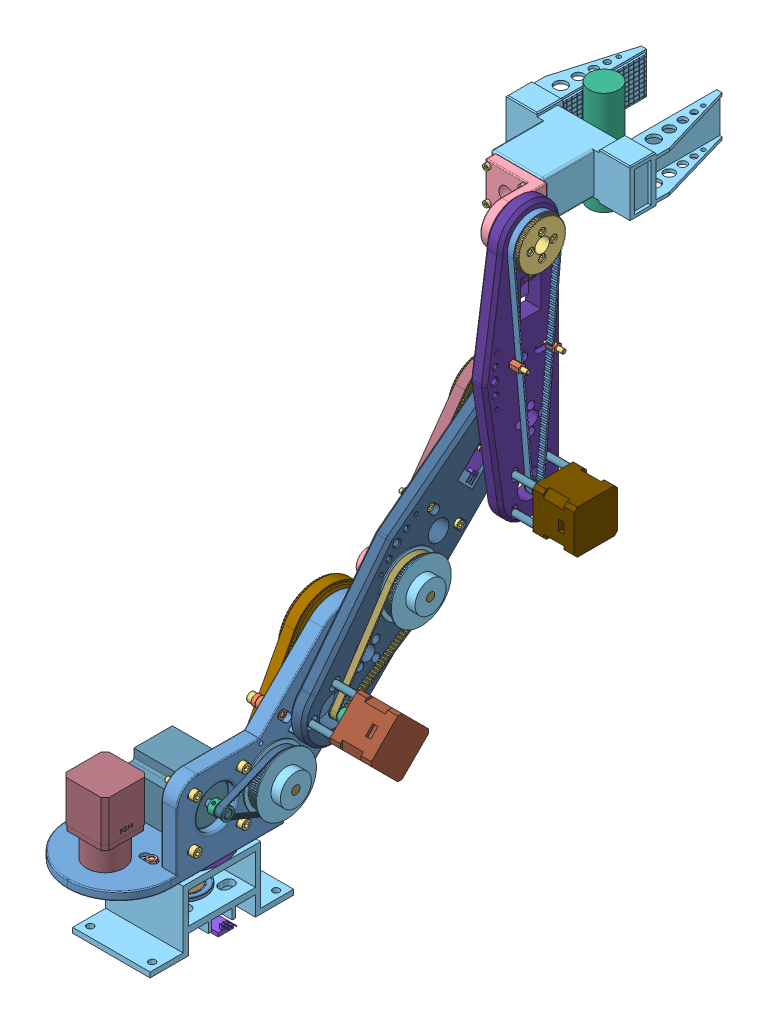
SolidWorks assembly R4 assem home axis, configuration Default. Lengths in mm.
Overall size (201 534.19 555.69).
175 component instances, 42 part files, 380 mates.
Components (placement in the parent):
- arm1-1: arm1 [Default] at (0 22.25 32) x (0 0 1) z (0 1 0) size (257.74 100 155.28)
- bearingCover-1: bearingCover [Default] at (50 142.4912 -110.7437) x (0 -0.707107 -0.707107) z (1 0 0) size (32 32 3)
- shaftJ1-1: shaftJ1 [Default] at (0 -34.75 0) x (0 0 -1) z (1 0 0) size (50 69 50)
- Pulleyhtd3m20Tbore8-1: Pulleyhtd3m20Tbore8 [Default] at (0 12.5 75.6) x (1 0 0) z (0 -1 0) size (22 22 24)
- pulley2GT80T-1: pulley2GT80T [Default] at (57.6 67.75 -36.0025) x (0 -0.778145 -0.628085) z (1 0 0) size (58 58 22)
- pulley2GT16Tbore6.35-1: pulley2GT16Tbore6.35 [Default] at (56.1 67.75 17.0975) x (0 0.483708 -0.87523) z (1 0 0) size (12.2 12.2 14)
- PulleyHTD3m15Tbore8-1: PulleyHTD3m15Tbore8 [Default] at (26.5 67.75 -36.0025) x (0 0.57686 0.816843) z (1 0 0) size (14 14 19.5)
- BeltHTD3m312L20T80T-1: BeltHTD3m312L20T80T [Default] at (0 12.5 0) x (0 0 1) z (0 1 0) size (125.04 78.09 10)
- BeltHTD3m363L15T80T-1: BeltHTD3m363L15T80T [Default] at (26.5 142.4912 -110.7437) x (0 -0.707107 0.707107) z (-1 0 0) size (152.76 78.09 10)
- belt2GT210L-1: belt2GT210L [Default] at (56.1 67.75 17.0975) x (0 0 -1) z (1 0 0) size (84.41 51.68 6)
- MagneticSensorV2-2: MagneticSensorV2 [Default] at (45.9 115.6211 -83.8737) x (0 -0.707107 0.707107) z (1 0 0) size (31 15 9)
- shaft8x70-1: shaft8x70 [Default] at (73.1 67.75 -36.0025) x (0 0 1) z (-1 0 0) size (8 8 61)
- Nema17L40PG14-1: Nema17L40PG14 [Default] at (0 99.75 75.6) x (0 0 -1) z (0 -1 0) size (42 42 88.5)
- Nema23_57x57x56-2: Nema23_57x57x56 [Default] at (-12 67.75 17.0975) x (0 0 -1) z (1 0 0) size (57 57 73)
- BeltTensionSpacer-1: BeltTensionSpacer [Default] at (35 113.7119 -46.6091) x (0 -0.41678 -0.909008) z (-1 0 0) size (6.4 6.4 3)
- BeltTensionSpacer-2: BeltTensionSpacer [Default] at (35 78.3566 -81.9645) x (0 -0.41678 -0.909008) z (-1 0 0) size (6.4 6.4 3)
- BeltTensionSpacer-6: BeltTensionSpacer [Default] at (-24.5 19.25 55) x (0.999608 0 0.027999) z (0 1 0) size (6.4 6.4 3)
- BeltTensionSpacer-5: BeltTensionSpacer [Default] at (24.5 22.25 55) x (0.852155 0 0.52329) z (0 -1 0) size (6.4 6.4 3)
- Washer45x60x1-2: Washer45x60x1 [5909K79] at (0 22.25 0) x (0 -1 0) z (0.730209 0 -0.683224) size (1 65 65)
- Washer45x60x1-1: Washer45x60x1 [5909K79] at (0 18.3 0) x (0 -1 0) z (0.528749 0 -0.848778) size (1 65 65)
- NeedleThrustBearing5909_45x60x3-1: NeedleThrustBearing5909_45x60x3 [5909K19] at (0 20.275 0) x (0.862783 0 0.505574) z (0.505574 0 -0.862783) size (65 3 65)
- bearing608 8x22x7-1: bearing608 8x22x7 [Default] at (50 67.75 -36.0025) x (0 -0.065699 -0.997839) z (0 0.997839 -0.065699) size (22 7 22)
- bearing608 8x22x7-2: bearing608 8x22x7 [Default] at (35 67.75 -36.0025) x (0 -0.995759 -0.092005) z (0 -0.092005 0.995759) size (22 7 22)
- bearing6806 30x42x7-3: bearing6806 30x42x7 [5972K282] at (38.5 142.4912 -110.7437) x (0 0.778145 0.628085) z (1 0 0) size (42 42 7)
- bearing6806 30x42x7-4: bearing6806 30x42x7 [5972K282] at (46.5 142.4912 -110.7437) x (0 -0.232241 -0.972658) z (-1 0 0) size (42 42 7)
- Bearing105 5x10x4-1: Bearing105 5x10x4 [7804K106] at (30 113.7119 -46.6091) x (0 0.558787 -0.829311) z (-1 0 0) size (10 10 4)
- Bearing105 5x10x4-4: Bearing105 5x10x4 [7804K106] at (26.1 78.3566 -81.9645) x (0 -0.623411 0.781894) z (-1 0 0) size (10 10 4)
- Bearing105 5x10x4-9: Bearing105 5x10x4 [7804K106] at (24.5 17.25 55) x (0.890608 0 -0.454771) z (0 -1 0) size (10 10 4)
- Bearing105 5x10x4-10: Bearing105 5x10x4 [7804K106] at (24.5 13.25 55) x (0.890608 0 -0.454771) z (0 -1 0) size (10 10 4)
- Bearing105 5x10x4-11: Bearing105 5x10x4 [7804K106] at (-24.5 13.25 55) x (-0.374722 0 0.927137) z (0 1 0) size (10 10 4)
- Bearing105 5x10x4-12: Bearing105 5x10x4 [7804K106] at (-24.5 17.25 55) x (0.156116 0 0.987739) z (0 1 0) size (10 10 4)
- Bearing105 5x10x4-2: Bearing105 5x10x4 [7804K106] at (26 113.7119 -46.6091) x (0 -0.774653 -0.632387) z (-1 0 0) size (10 10 4)
- Bearing105 5x10x4-3: Bearing105 5x10x4 [7804K106] at (30.1 78.3566 -81.9645) x (0 -0.931032 -0.364937) z (1 0 0) size (10 10 4)
- socket head cap screw_iso0-13: socket head cap screw_iso0 [ISO 4762 M4 x 12 - 12N] at (0 38.25 20) x (0 -1 0) z (0 0 1) size (16 7 7)
- socket head cap screw_iso0-14: socket head cap screw_iso0 [ISO 4762 M4 x 12 - 12N] at (20 38.25 0) x (0 -1 0) z (0 0 1) size (16 7 7)
- socket head cap screw_iso0-15: socket head cap screw_iso0 [ISO 4762 M4 x 12 - 12N] at (0 38.25 -20) x (0 -1 0) z (0 0 1) size (16 7 7)
- socket head cap screw_iso0-16: socket head cap screw_iso0 [ISO 4762 M4 x 12 - 12N] at (-20 38.25 0) x (0 -1 0) z (0 0 1) size (16 7 7)
- hex nut style 1 gradeab_iso00-1: hex nut style 1 gradeab_iso00 [ISO - 4032 - M5 - W - N] at (49.7 113.7119 -46.6091) x (0 -0.707107 0.707107) z (1 0 0) size (8 9.24 4.7)
- hex nut style 1 gradeab_iso00-2: hex nut style 1 gradeab_iso00 [ISO - 4032 - M5 - W - N] at (49.7 78.3566 -81.9645) x (0 0.965926 0.258819) z (1 0 0) size (8 9.24 4.7)
- socket head cap screw_iso0-20: socket head cap screw_iso0 [ISO 4762 M5 x 25 - 25N] at (19 113.7119 -46.6091) size (30 8.5 8.5)
- socket head cap screw_iso0-21: socket head cap screw_iso0 [ISO 4762 M5 x 25 - 25N] at (19.1 78.3566 -81.9645) size (30 8.5 8.5)
- socket head cap screw_iso0-57: socket head cap screw_iso0 [ISO 4762 M5 x 20 - 20N] at (24.5 6.25 55) x (0 1 0) z (0 0 1) size (25 8.5 8.5)
- socket head cap screw_iso0-58: socket head cap screw_iso0 [ISO 4762 M5 x 20 - 20N] at (-24.5 6.25 55) x (0 1 0) z (0 0 1) size (25 8.5 8.5)
- hex nut style 1 gradeab_iso00-15: hex nut style 1 gradeab_iso00 [ISO - 4032 - M5 - W - N] at (-24.5 31.95 55) x (-0.866025 0 0.5) z (0 1 0) size (8 9.24 4.7)
- hex nut style 1 gradeab_iso00-16: hex nut style 1 gradeab_iso00 [ISO - 4032 - M5 - W - N] at (24.5 31.95 55) x (-0.866025 0 -0.5) z (0 1 0) size (8 9.24 4.7)
- socket head cap screw_iso0-80: socket head cap screw_iso0 [ISO 4762 M2 x 12 - 12N] at (51.4 117.7424 -93.066) x (-1 0 0) z (0 0.924225 0.381849) size (14 3.8 3.8)
- socket head cap screw_iso0-81: socket head cap screw_iso0 [ISO 4762 M2 x 12 - 12N] at (51.4 124.8135 -85.995) x (-1 0 0) z (0 0.924225 0.381849) size (14 3.8 3.8)
- hex nut style 1 gradeab_iso00-25: hex nut style 1 gradeab_iso00 [ISO - 4032 - M2 - W - N] at (37.4 117.7424 -93.066) x (0 0 1) z (-1 0 0) size (4 4.62 1.6)
- hex nut style 1 gradeab_iso00-26: hex nut style 1 gradeab_iso00 [ISO - 4032 - M2 - W - N] at (37.4 124.8135 -85.995) x (0 0 1) z (-1 0 0) size (4 4.62 1.6)
- socket head cap screw_iso0-96: socket head cap screw_iso0 [ISO 4762 M5 x 25 - 25N] at (55 91.32 40.6675) x (-1 0 0) z (0 -0.924225 -0.381849) size (30 8.5 8.5)
- socket head cap screw_iso0-97: socket head cap screw_iso0 [ISO 4762 M5 x 25 - 25N] at (55 91.32 -6.4725) x (-1 0 0) z (0 -0.924225 -0.381849) size (30 8.5 8.5)
- socket head cap screw_iso0-98: socket head cap screw_iso0 [ISO 4762 M5 x 25 - 25N] at (55 44.18 -6.4725) x (-1 0 0) z (0 -0.924225 -0.381849) size (30 8.5 8.5)
- socket head cap screw_iso0-99: socket head cap screw_iso0 [ISO 4762 M5 x 25 - 25N] at (55 44.18 40.6675) x (-1 0 0) z (0 -0.924225 -0.381849) size (30 8.5 8.5)
- socket head cap screw_iso0-104: socket head cap screw_iso0 [ISO 4762 M3 x 12 - 12N] at (9.8995 19.25 85.4995) x (0 1 0) z (0 0 1) size (15 5.5 5.5)
- socket head cap screw_iso0-105: socket head cap screw_iso0 [ISO 4762 M3 x 12 - 12N] at (9.8995 19.25 65.7005) x (0 1 0) z (0 0 1) size (15 5.5 5.5)
- socket head cap screw_iso0-106: socket head cap screw_iso0 [ISO 4762 M3 x 12 - 12N] at (-9.8995 19.25 85.4995) x (0 1 0) z (0 0 1) size (15 5.5 5.5)
- socket head cap screw_iso0-107: socket head cap screw_iso0 [ISO 4762 M3 x 12 - 12N] at (-9.8995 19.25 65.7005) x (0 1 0) z (0 0 1) size (15 5.5 5.5)
- hex nut style 1 gradeab_iso00-35: hex nut style 1 gradeab_iso00 [ISO - 4032 - M5 - W - N] at (30.3 91.32 40.6675) x (0 0 1) z (-1 0 0) size (8 9.24 4.7)
- hex nut style 1 gradeab_iso00-36: hex nut style 1 gradeab_iso00 [ISO - 4032 - M5 - W - N] at (30.3 91.32 -6.4725) x (0 0 1) z (-1 0 0) size (8 9.24 4.7)
- hex nut style 1 gradeab_iso00-37: hex nut style 1 gradeab_iso00 [ISO - 4032 - M5 - W - N] at (30.3 44.18 -6.4725) x (0 0 1) z (-1 0 0) size (8 9.24 4.7)
- hex nut style 1 gradeab_iso00-38: hex nut style 1 gradeab_iso00 [ISO - 4032 - M5 - W - N] at (40.3966 44.18 40.6675) x (0 0 -1) z (1 0 0) size (8 9.24 4.7)
- base-1: base [Default] x (1 0 0) z (0 1 0) size (75 138.93 61)
- bearing6806 30x42x7-1: bearing6806 30x42x7 [5972K282] at (0 -30.5984 0) x (0.837169 0 0.546944) z (0 -1 0) size (42 42 7)
- pulleyHTD3m80Tbase-1: pulleyHTD3m80Tbase [Default] at (0 12 0) x (1 0 0) z (0 1 0) size (75.63 75.63 12)
- bearing6806 30x42x7-2: bearing6806 30x42x7 [5972K282] at (0 14.3 0) x (0.999895 0 -0.014508) z (0 1 0) size (42 42 7)
- shaftJ1endPlate-1: shaftJ1endPlate [Default] at (0 -34.75 0) x (0 0 -1) z (0 -1 0) size (40 40 6)
- MagneticSensor-3: MagneticSensor [Default] at (31.5 -49.5984 0) x (1 0 0) z (0 1 0) size (31 15 7.5)
- socket head cap screw_iso0-132: socket head cap screw_iso0 [ISO 4762 M5 x 16 - 16N] at (21 -5 -21) x (0 1 0) z (0 0 1) size (21 8.5 8.5)
- socket head cap screw_iso0-133: socket head cap screw_iso0 [ISO 4762 M5 x 16 - 16N] at (21 -5 21) x (0 1 0) z (0 0 1) size (21 8.5 8.5)
- socket head cap screw_iso0-134: socket head cap screw_iso0 [ISO 4762 M5 x 16 - 16N] at (-21 -5 21) x (0 1 0) z (0 0 1) size (21 8.5 8.5)
- socket head cap screw_iso0-135: socket head cap screw_iso0 [ISO 4762 M5 x 16 - 16N] at (-21 -5 -21) x (0 1 0) z (0 0 1) size (21 8.5 8.5)
- socket head cap screw_iso0-136: socket head cap screw_iso0 [ISO 4762 M3 x 16 - 16N] at (12.5 -43.75 0) x (0 1 0) z (0 0 1) size (19 5.5 5.5)
- socket head cap screw_iso0-137: socket head cap screw_iso0 [ISO 4762 M3 x 16 - 16N] at (0 -43.75 12.5) x (0 1 0) z (0 0 1) size (19 5.5 5.5)
- socket head cap screw_iso0-138: socket head cap screw_iso0 [ISO 4762 M3 x 16 - 16N] at (-12.5 -43.75 0) x (0 1 0) z (0 0 1) size (19 5.5 5.5)
- socket head cap screw_iso0-139: socket head cap screw_iso0 [ISO 4762 M3 x 16 - 16N] at (0 -43.75 -12.5) x (0 1 0) z (0 0 1) size (19 5.5 5.5)
- socket head cap screw_iso0-140: socket head cap screw_iso0 [ISO 4762 M2 x 12 - 12N] at (23.5 -51.5984 -5) x (0 1 0) z (-0.11823 0 0.992986) size (14 3.8 3.8)
- socket head cap screw_iso0-141: socket head cap screw_iso0 [ISO 4762 M2 x 12 - 12N] at (23.5 -51.5984 5) x (0 1 0) z (0 0 1) size (14 3.8 3.8)
- hex nut style 1 gradeab_iso00-59: hex nut style 1 gradeab_iso00 [ISO - 4032 - M2 - W - N] at (23.5 -40.9984 -5) x (1 0 0) z (0 1 0) size (4 4.62 1.6)
- hex nut style 1 gradeab_iso00-60: hex nut style 1 gradeab_iso00 [ISO - 4032 - M2 - W - N] at (23.5 -40.9984 5) x (1 0 0) z (0 1 0) size (4 4.62 1.6)
- socket head cap screw_iso0-142: socket head cap screw_iso0 [ISO 4762 M4 x 40 - 20N] at (19 134.713 -102.9655) size (44 7 7)
- socket head cap screw_iso0-143: socket head cap screw_iso0 [ISO 4762 M4 x 40 - 20N] at (19 134.713 -118.5219) size (44 7 7)
- socket head cap screw_iso0-144: socket head cap screw_iso0 [ISO 4762 M4 x 40 - 20N] at (19 150.2694 -118.5219) size (44 7 7)
- socket head cap screw_iso0-145: socket head cap screw_iso0 [ISO 4762 M4 x 40 - 20N] at (19 150.2694 -102.9655) size (44 7 7)
- PulleyHtd3m80Tbore8-2: PulleyHtd3m80Tbore8 [Default] at (25.5 142.4912 -110.7437) x (0 -0.707107 -0.707107) z (1 0 0) size (75.96 75.93 32)
- arm2-1: arm2 [Default] at (60.5 110.6714 -78.9239) x (0 0.707107 -0.707107) z (1 0 0) size (300.08 74.89 15.27)
- bearing6806 30x42x7-5: bearing6806 30x42x7 [5972K282] at (64.5 280.4336 -248.6861) x (0 -0.073672 -0.997283) z (1 0 0) size (42 42 7)
- bearing6806 30x42x7-6: bearing6806 30x42x7 [5972K282] at (56.5 280.4336 -248.6861) x (0 -0.383049 0.923728) z (-1 0 0) size (42 42 7)
- bearing608 8x22x7-3: bearing608 8x22x7 [Default] at (68 181.3255 -149.578) x (0 0 -1) z (0 1 0) size (22 7 22)
- bearing608 8x22x7-4: bearing608 8x22x7 [Default] at (60 181.3255 -149.578) x (0 0 -1) z (0 1 0) size (22 7 22)
- nema17L48arm2-1: nema17L48arm2 [Défaut] at (111 140.3699 -78.9239) x (-1 0 0) z (0 0.707107 -0.707107) size (63 42 42)
- pulley2GT16Tbore6.35-2: pulley2GT16Tbore6.35 [Default] at (72.5 110.6714 -78.9239) x (0 0.383049 -0.923728) z (-1 0 0) size (12.2 12.2 14)
- pulley2GT80T-2: pulley2GT80T [Default] at (74.5 181.3255 -149.578) x (0 -0.954986 -0.296652) z (1 0 0) size (58 58 22)
- belt2GTarm2-1: belt2GTarm2 [Default] at (72 110.6714 -78.9239) x (0 0.707107 -0.707107) z (1 0 0) size (131.74 52.19 6)
- shaft8x70-2: shaft8x70 [Default] at (29 181.3255 -149.578) x (0 0.563863 -0.825868) z (1 0 0) size (8 8 61)
- Pulleyhtd3m20Tbore8-2: Pulleyhtd3m20Tbore8 [Default] at (46.5 181.3255 -149.578) x (0 0 -1) z (1 0 0) size (22 22 24)
- beltHTD3marm2-1: beltHTD3marm2 [Default] at (47 280.4336 -248.6861) x (0 -0.707107 0.707107) z (1 0 0) size (184.35 67.59 10)
- MagneticSensor-6: MagneticSensor [Default] at (63 250.028 -218.2805) x (0 -0.707107 0.707107) z (1 0 0) size (31 15 7.5)
- cover nuts-1: cover nuts [Default] at (68 110.6714 -56.2965) x (0 -0.818287 -0.57481) z (1 0 0) size (6 6 23)
- cover nuts-2: cover nuts [Default] at (68 133.2988 -78.9239) x (0 0.708033 -0.706179) z (1 0 0) size (6 6 23)
- cover nuts-3: cover nuts [Default] at (68 88.044 -78.9239) x (0 -0.829446 -0.558587) z (1 0 0) size (6 6 23)
- cover nuts-4: cover nuts [Default] at (91 110.6714 -101.5513) x (0 0 1) z (-1 0 0) size (6 6 23)
- hex thin nut chamfered gradeab_iso-2: hex thin nut chamfered gradeab_iso [ISO - 4035 - M4 - N] at (50.8 233.411 -172.6721) x (0 0 1) z (-1 0 0) size (7 8.08 2.2)
- hex thin nut chamfered gradeab_iso-3: hex thin nut chamfered gradeab_iso [ISO - 4035 - M4 - N] at (48.6 233.411 -172.6721) x (0 0 1) z (-1 0 0) size (7 8.08 2.2)
- hex thin nut chamfered gradeab_iso-4: hex thin nut chamfered gradeab_iso [ISO - 4035 - M4 - N] at (46.4 233.411 -172.6721) x (0 0 1) z (-1 0 0) size (7 8.08 2.2)
- hex thin nut chamfered gradeab_iso-5: hex thin nut chamfered gradeab_iso [ISO - 4035 - M4 - N] at (44.2 233.411 -172.6721) x (0 0 1) z (-1 0 0) size (7 8.08 2.2)
- hex thin nut chamfered gradeab_iso-6: hex thin nut chamfered gradeab_iso [ISO - 4035 - M4 - N] at (42 233.411 -172.6721) x (0 0 1) z (-1 0 0) size (7 8.08 2.2)
- hex thin nut chamfered gradeab_iso-7: hex thin nut chamfered gradeab_iso [ISO - 4035 - M4 - N] at (50.8 204.4196 -201.6635) x (0 0 1) z (-1 0 0) size (7 8.08 2.2)
- hex thin nut chamfered gradeab_iso-8: hex thin nut chamfered gradeab_iso [ISO - 4035 - M4 - N] at (48.6 204.4196 -201.6635) x (0 0 1) z (-1 0 0) size (7 8.08 2.2)
- hex thin nut chamfered gradeab_iso-9: hex thin nut chamfered gradeab_iso [ISO - 4035 - M4 - N] at (46.4 204.4196 -201.6635) x (0 0 1) z (-1 0 0) size (7 8.08 2.2)
- hex thin nut chamfered gradeab_iso-10: hex thin nut chamfered gradeab_iso [ISO - 4035 - M4 - N] at (44.2 204.4196 -201.6635) x (0 0 1) z (-1 0 0) size (7 8.08 2.2)
- hex thin nut chamfered gradeab_iso-11: hex thin nut chamfered gradeab_iso [ISO - 4035 - M4 - N] at (42 204.4196 -201.6635) x (0 0 1) z (-1 0 0) size (7 8.08 2.2)
- hex thin nut chamfered gradeab_iso-12: hex thin nut chamfered gradeab_iso [ISO - 4035 - M2 - N] at (64.2 259.2204 -220.4018) x (0 0 -1) z (1 0 0) size (4 4.62 1.2)
- hex thin nut chamfered gradeab_iso-13: hex thin nut chamfered gradeab_iso [ISO - 4035 - M2 - N] at (64.2 252.1493 -227.4729) x (0 0 -1) z (1 0 0) size (4 4.62 1.2)
- socket head cap screw_iso0-174: socket head cap screw_iso0 [ISO 4762 M3 x 30 - 18N] at (55 110.6714 -56.2965) size (33 5.5 5.5)
- socket head cap screw_iso0-175: socket head cap screw_iso0 [ISO 4762 M3 x 30 - 18N] at (55 133.2988 -78.9239) size (33 5.5 5.5)
- socket head cap screw_iso0-176: socket head cap screw_iso0 [ISO 4762 M3 x 30 - 18N] at (55 88.044 -78.9239) x (1 0 0) z (0 -0.320522 -0.947241) size (33 5.5 5.5)
- socket head cap screw_iso0-177: socket head cap screw_iso0 [ISO 4762 M3 x 30 - 18N] at (55 110.6714 -101.5513) size (33 5.5 5.5)
- socket head cap screw_iso0-189: socket head cap screw_iso0 [ISO 4762 M4 x 25 - 25N] at (67 233.411 -172.6721) x (-1 0 0) z (0 0.247798 0.968812) size (29 7 7)
- socket head cap screw_iso0-190: socket head cap screw_iso0 [ISO 4762 M4 x 25 - 25N] at (67 204.4196 -201.6635) x (-1 0 0) z (0 -0.924225 -0.381849) size (29 7 7)
- socket head cap screw_iso0-191: socket head cap screw_iso0 [ISO 4762 M2 x 10 - 10N] at (68.5 259.2204 -220.4018) x (-1 0 0) z (0 0.924225 0.381849) size (12 3.8 3.8)
- socket head cap screw_iso0-192: socket head cap screw_iso0 [ISO 4762 M2 x 10 - 10N] at (68.5 252.1493 -227.4729) x (-1 0 0) z (0 0.924225 0.381849) size (12 3.8 3.8)
- hex thin nut chamfered gradeab_iso-14: hex thin nut chamfered gradeab_iso [ISO - 4035 - M2 - N] at (56.8 259.2204 -220.4018) x (0 0 1) z (-1 0 0) size (4 4.62 1.2)
- hex thin nut chamfered gradeab_iso-15: hex thin nut chamfered gradeab_iso [ISO - 4035 - M2 - N] at (56.8 252.1493 -227.4729) x (0 0 1) z (-1 0 0) size (4 4.62 1.2)
- socket head cap screw_iso0-193: socket head cap screw_iso0 [ISO 4762 M4 x 40 - 20N] at (39 269.4336 -248.6861) size (44 7 7)
- socket head cap screw_iso0-194: socket head cap screw_iso0 [ISO 4762 M4 x 40 - 20N] at (39 291.4336 -248.6861) size (44 7 7)
- socket head cap screw_iso0-195: socket head cap screw_iso0 [ISO 4762 M4 x 40 - 20N] at (39 280.4336 -237.6861) size (44 7 7)
- socket head cap screw_iso0-196: socket head cap screw_iso0 [ISO 4762 M4 x 40 - 20N] at (39 280.4336 -259.6861) size (44 7 7)
- PulleyHtd3m80Tbore8arm2-1: PulleyHtd3m80Tbore8arm2 [Default] at (45.5 280.4336 -248.6861) x (0 0 -1) z (1 0 0) size (63.51 63.51 32)
- bearingCover-2: bearingCover [Default] at (73 280.4336 -248.6861) x (0 -1 0) z (-1 0 0) size (32 32 3)
- arm3-1: arm3 [Default] at (80.5 225.4336 -248.6861) x (0 1 0) z (1 0 0) size (265.75 74.89 15.27)
- bearing6806 30x42x7-7: bearing6806 30x42x7 [5972K282] at (84.5 431.1836 -248.6861) x (0 0 -1) z (1 0 0) size (42 42 7)
- bearing6806 30x42x7-8: bearing6806 30x42x7 [5972K282] at (76.5 431.1836 -248.6861) x (0 0 -1) z (1 0 0) size (42 42 7)
- nema17L48arm3-1: nema17L48arm3 [Défaut] at (131 246.4336 -227.6861) x (-1 0 0) z (0 1 0) size (63 42 42)
- pulley2GT16Tbore6.35-3: pulley2GT16Tbore6.35 [Default] at (92.5 225.4336 -248.6861) x (0 0.383049 -0.923728) z (-1 0 0) size (12.2 12.2 14)
- belt2GTarm3-1: belt2GTarm3 [Default] at (92 431.1836 -248.6861) x (0 -1 0) z (1 0 0) size (235.46 47.53 6)
- MagneticSensor-4: MagneticSensor [Default] at (78 386.1836 -248.6861) x (0 -1 0) z (-1 0 0) size (31 15 7.5)
- cover nuts-5: cover nuts [Default] at (88 209.4336 -232.6861) x (0 -0.924225 -0.381849) z (1 0 0) size (6 6 23)
- cover nuts-6: cover nuts [Default] at (88 241.4336 -232.6861) x (0 -0.921224 -0.389031) z (1 0 0) size (6 6 23)
- cover nuts-7: cover nuts [Default] at (88 209.4336 -264.6861) x (0 -0.923758 -0.382976) z (1 0 0) size (6 6 23)
- cover nuts-8: cover nuts [Default] at (88 241.4336 -264.6861) x (0 -0.832631 -0.553828) z (1 0 0) size (6 6 23)
- socket head cap screw_iso0-197: socket head cap screw_iso0 [ISO 4762 M2 x 10 - 10N] at (72.5 394.1836 -243.6861) size (12 3.8 3.8)
- socket head cap screw_iso0-198: socket head cap screw_iso0 [ISO 4762 M2 x 10 - 10N] at (72.5 394.1836 -253.6861) size (12 3.8 3.8)
- hex thin nut gradeb_iso00-2: hex thin nut gradeb_iso00 [ISO - 4036 - M2 - N] at (84.2 394.1836 -243.6861) x (0 0 -1) z (1 0 0) size (4 4.62 1.2)
- hex thin nut gradeb_iso00-3: hex thin nut gradeb_iso00 [ISO - 4036 - M2 - N] at (84.2 394.1836 -253.6861) x (0 0 -1) z (1 0 0) size (4 4.62 1.2)
- hex thin nut gradeb_iso00-4: hex thin nut gradeb_iso00 [ISO - 4036 - M4 - N] at (90.2 334.9698 -231.3738) x (0 0 -1) z (1 0 0) size (7 8.08 2.2)
- hex thin nut gradeb_iso00-5: hex thin nut gradeb_iso00 [ISO - 4036 - M4 - N] at (92.4 334.9698 -231.3738) x (0 0 -1) z (1 0 0) size (7 8.08 2.2)
- hex thin nut gradeb_iso00-6: hex thin nut gradeb_iso00 [ISO - 4036 - M4 - N] at (94.6 334.9698 -231.3738) x (0 0 -1) z (1 0 0) size (7 8.08 2.2)
- hex thin nut gradeb_iso00-7: hex thin nut gradeb_iso00 [ISO - 4036 - M4 - N] at (96.8 334.9698 -231.3738) x (0 0 -1) z (1 0 0) size (7 8.08 2.2)
- hex thin nut gradeb_iso00-8: hex thin nut gradeb_iso00 [ISO - 4036 - M4 - N] at (90.2 334.9698 -266.1861) x (0 0 -1) z (1 0 0) size (7 8.08 2.2)
- hex thin nut gradeb_iso00-9: hex thin nut gradeb_iso00 [ISO - 4036 - M4 - N] at (92.4 334.9698 -266.1861) x (0 0 -1) z (1 0 0) size (7 8.08 2.2)
- hex thin nut gradeb_iso00-10: hex thin nut gradeb_iso00 [ISO - 4036 - M4 - N] at (94.6 334.9698 -266.1861) x (0 0 -1) z (1 0 0) size (7 8.08 2.2)
- hex thin nut gradeb_iso00-11: hex thin nut gradeb_iso00 [ISO - 4036 - M4 - N] at (96.8 334.9698 -266.1861) x (0 0 -1) z (1 0 0) size (7 8.08 2.2)
- socket head cap screw_iso0-199: socket head cap screw_iso0 [ISO 4762 M3 x 30 - 18N] at (75 209.4336 -232.6861) size (33 5.5 5.5)
- socket head cap screw_iso0-200: socket head cap screw_iso0 [ISO 4762 M3 x 30 - 18N] at (75 241.4336 -232.6861) size (33 5.5 5.5)
- socket head cap screw_iso0-201: socket head cap screw_iso0 [ISO 4762 M3 x 30 - 18N] at (75 209.4336 -264.6861) x (1 0 0) z (0 -0.331782 0.943356) size (33 5.5 5.5)
- socket head cap screw_iso0-202: socket head cap screw_iso0 [ISO 4762 M3 x 30 - 18N] at (75 241.4336 -264.6861) x (1 0 0) z (0 -0.017552 0.999846) size (33 5.5 5.5)
- socket head cap screw_iso0-203: socket head cap screw_iso0 [ISO 4762 M4 x 25 - 25N] at (74 334.9698 -231.3738) x (1 0 0) z (0 0.99119 0.132448) size (29 7 7)
- socket head cap screw_iso0-204: socket head cap screw_iso0 [ISO 4762 M4 x 25 - 25N] at (74 334.9698 -266.1861) x (1 0 0) z (0 -0.279125 0.960255) size (29 7 7)
- pulley2GT60T-1: pulley2GT60T [Default] at (93.5 431.1836 -248.6861) x (0 0 1) z (-1 0 0) size (45.3 45.3 27)
- gripper holder-1: gripper holder [Default] at (64 431.1836 -248.6861) x (0 0 -1) z (1 0 0) size (55 40 50)
- Part1g-1: Part1g [Default] at (39.0001 431.1835 -283.6861) x (1 -0.000137 0) z (0 0 1) size (120 46 160)
- payload-1: payload [Default] at (39.493 379.1834 -368.0651) x (0.990185 -0.000136 -0.139766) z (0.000137 1 0) size (28.76 28.76 100)
- bearingCover-3: bearingCover [Default] at (72 431.1836 -248.6861) x (0 -1 0) z (-1 0 0) size (32 32 3)
- hex thin nut gradeb_iso00-12: hex thin nut gradeb_iso00 [ISO - 4036 - M4 - N] at (56.8 442.1836 -248.6861) x (0 0 1) z (-1 0 0) size (7 8.08 2.2)
- hex thin nut gradeb_iso00-13: hex thin nut gradeb_iso00 [ISO - 4036 - M4 - N] at (56.8 420.1836 -248.6861) x (0 0 1) z (-1 0 0) size (7 8.08 2.2)
- hex thin nut gradeb_iso00-14: hex thin nut gradeb_iso00 [ISO - 4036 - M4 - N] at (56.8 431.1836 -237.6861) x (0 0 1) z (-1 0 0) size (7 8.08 2.2)
- hex thin nut gradeb_iso00-15: hex thin nut gradeb_iso00 [ISO - 4036 - M4 - N] at (56.8 431.1836 -259.6861) x (0 0 1) z (-1 0 0) size (7 8.08 2.2)
- socket head cap screw_iso0-205: socket head cap screw_iso0 [ISO 4762 M3 x 20 - 20N] at (56.22 446.6859 -270.6861) x (0 0 -1) z (0.996957 -0.077948 0) size (23 5.5 5.5)
- socket head cap screw_iso0-206: socket head cap screw_iso0 [ISO 4762 M3 x 20 - 20N] at (21.78 415.6813 -270.6861) x (0 0 -1) z (0.996957 -0.077948 0) size (23 5.5 5.5)
- socket head cap screw_iso0-207: socket head cap screw_iso0 [ISO 4762 M3 x 20 - 20N] at (21.78 446.6859 -270.6861) x (0 0 -1) z (0.996957 -0.077948 0) size (23 5.5 5.5)
- socket head cap screw_iso0-208: socket head cap screw_iso0 [ISO 4762 M3 x 20 - 20N] at (56.22 415.6813 -270.6861) x (0 0 -1) z (0.996957 -0.077948 0) size (23 5.5 5.5)
- socket head cap screw_iso0-209: socket head cap screw_iso0 [ISO 4762 M4 x 35 - 20N] at (98 442.1836 -248.6861) x (-1 0 0) z (0 0.924225 0.381849) size (39 7 7)
- socket head cap screw_iso0-210: socket head cap screw_iso0 [ISO 4762 M4 x 35 - 20N] at (98 420.1836 -248.6861) x (-1 0 0) z (0 0.924225 0.381849) size (39 7 7)
- socket head cap screw_iso0-211: socket head cap screw_iso0 [ISO 4762 M4 x 35 - 20N] at (98 431.1836 -237.6861) x (-1 0 0) z (0 0.924225 0.381849) size (39 7 7)
- socket head cap screw_iso0-212: socket head cap screw_iso0 [ISO 4762 M4 x 35 - 20N] at (98 431.1836 -259.6861) x (-1 0 0) z (0 0.924225 0.381849) size (39 7 7)
Mates (geometry in assembly coordinates):
- Fix J1: parallel aligned: plane of base-1 through (37.5 6 37.5) normal (1 0 0); plane of arm1-1 through (50 30.25 -48) normal (1 0 0)
- Concentric1: concentric aligned: cylinder of base-1 through (0 29.44 0) axis (0 -1 0) radius 21.05; cylinder of bearing6806 30x42x7-1 through (0 -34.0984 0) axis (0 -1 0) radius 21
- Coincident1: coincident anti-aligned: plane of base-1 through (0 -34.0984 0) normal (0 1 0); plane of bearing6806 30x42x7-1 through (-11.2944 -34.0984 17.2875) normal (0 -1 0)
- Concentric2: concentric anti-aligned: cylinder of base-1 through (0 6 0) axis (0 -1 0) radius 16; cylinder of pulleyHTD3m80Tbase-1 through (0 10.8 0) axis (0 1 0) radius 21.05
- Concentric3: concentric anti-aligned: cylinder of base-1 through (21 6 21) axis (0 -1 0) radius 2.75; cylinder of pulleyHTD3m80Tbase-1 through (21 6 21) axis (0 1 0) radius 3
- Coincident2: coincident anti-aligned: plane of base-1 through (0 6 0) normal (0 1 0); plane of pulleyHTD3m80Tbase-1 through (0 6 0) normal (0 -1 0)
- Concentric4: concentric aligned: cylinder of base-1 through (21 6 -21) axis (0 -1 0) radius 2.75; cylinder of socket head cap screw_iso-1 through (21 -36.75 -21) axis (0 -1 0) radius 4.25
- Coincident3: coincident anti-aligned: plane of base-1 through (0 0 0) normal (0 -1 0); plane of socket head cap screw_iso-1 through (16.75 0 -21) normal (0 1 0)
- Concentric5: concentric aligned: cylinder of base-1 through (21 6 21) axis (0 -1 0) radius 2.75; cylinder of socket head cap screw_iso-2 through (21 -36.75 21) axis (0 -1 0) radius 4.25
- Coincident4: coincident anti-aligned: plane of base-1 through (0 0 0) normal (0 -1 0); plane of socket head cap screw_iso-2 through (16.75 0 21) normal (0 1 0)
- Concentric6: concentric aligned: cylinder of base-1 through (-21 6 21) axis (0 -1 0) radius 2.75; cylinder of socket head cap screw_iso-3 through (-21 -36.75 21) axis (0 -1 0) radius 4.25
- Coincident5: coincident anti-aligned: plane of base-1 through (0 0 0) normal (0 -1 0); plane of socket head cap screw_iso-3 through (-25.25 0 21) normal (0 1 0)
- Concentric7: concentric aligned: cylinder of base-1 through (-21 6 -21) axis (0 -1 0) radius 2.75; cylinder of socket head cap screw_iso-4 through (-21 -36.75 -21) axis (0 -1 0) radius 4.25
- Coincident6: coincident anti-aligned: plane of base-1 through (0 0 0) normal (0 -1 0); plane of socket head cap screw_iso-4 through (-25.25 0 -21) normal (0 1 0)
- Concentric8: concentric aligned: cylinder of pulleyHTD3m80Tbase-1 through (0 10.8 0) axis (0 1 0) radius 21.05; cylinder of bearing6806 30x42x7-2 through (0 17.8 0) axis (0 1 0) radius 21
- Coincident7: coincident anti-aligned: plane of pulleyHTD3m80Tbase-1 through (0 10.8 0) normal (0 1 0); plane of bearing6806 30x42x7-2 through (-0.2996 10.8 -20.6478) normal (0 -1 0)
- Concentric9: concentric aligned: cylinder of pulleyHTD3m80Tbase-1 through (0 10.8 0) axis (0 1 0) radius 21.05; cylinder of Washer45x60x1-1 through (0 17.8 0) axis (0 1 0) radius 32.5
- Coincident8: coincident anti-aligned: plane of pulleyHTD3m80Tbase-1 through (0 17.8 0) normal (0 1 0); plane of Washer45x60x1-1 through (0 17.8 0) normal (0 -1 0)
- Concentric10: concentric anti-aligned: cylinder of pulleyHTD3m80Tbase-1 through (0 10.8 0) axis (0 1 0) radius 21.05; cylinder of NeedleThrustBearing5909_45x60x3-1 through (0 18.775 0) axis (0 -1 0) radius 32.5
- Distance1: distance = 0.2 mm anti-aligned: plane of NeedleThrustBearing5909_45x60x3-1 through (-16.4311 19 28.0405) normal (0 -1 0); plane of Washer45x60x1-1 through (0 18.8 0) normal (0 1 0)
- Concentric11: concentric aligned: cylinder of pulleyHTD3m80Tbase-1 through (0 10.8 0) axis (0 1 0) radius 21.05; cylinder of Washer45x60x1-2 through (0 21.75 0) axis (0 1 0) radius 22.525
- Distance2: distance = 0.2 mm anti-aligned: plane of NeedleThrustBearing5909_45x60x3-1 through (-16.2626 21.55 27.7529) normal (0 1 0); plane of Washer45x60x1-2 through (0 21.75 0) normal (0 -1 0)
- Concentric12: concentric aligned: cylinder of base-1 through (0 6 0) axis (0 -1 0) radius 16; cylinder of arm1-1 through (0 30.25 0) axis (0 -1 0) radius 15.5
- Coincident12: coincident anti-aligned: plane of arm1-1 through (0 22.75 0) normal (0 -1 0); plane of Washer45x60x1-2 through (0 22.75 0) normal (0 1 0)
- Concentric15: concentric anti-aligned: cylinder of arm1-1 through (0 30.25 75.6) axis (0 -1 0) radius 11.5; cylinder of Nema17L40PG14-1 through (0 30.25 75.6) axis (0 1 0) radius 18
- Concentric16: concentric aligned: cylinder of arm1-1 through (-9.8995 30.25 85.4995) axis (0 -1 0) radius 1.65; cylinder of Nema17L40PG14-1 through (-9.8995 38.25 85.4995) axis (0 -1 0) radius 2
- Coincident16: coincident anti-aligned: plane of arm1-1 through (0 30.25 32) normal (0 1 0); plane of Nema17L40PG14-1 through (0 30.25 75.6) normal (0 -1 0)
- Concentric20: concentric anti-aligned: cylinder of Nema17L40PG14-1 through (0 11.25 75.6) axis (0 1 0) radius 4; cylinder of Pulleyhtd3m20Tbore8-1 through (0 30 75.6) axis (0 -1 0) radius 11
- Coincident17: coincident anti-aligned: plane of pulleyHTD3m80Tbase-1 through (0 18 0) normal (0 1 0); plane of Pulleyhtd3m20Tbore8-1 through (0 18 75.6) normal (0 -1 0)
- Concentric21: concentric aligned: cylinder of NeedleThrustBearing5909_45x60x3-1 through (0 18.775 0) axis (0 -1 0) radius 32.5; cylinder of BeltHTD3m312L20T80T-1 through (0 17.5 0) axis (0 -1 0) radius 39.0462
- Concentric22: concentric aligned: cylinder of Pulleyhtd3m20Tbore8-1 through (0 30 75.6) axis (0 -1 0) radius 11; cylinder of BeltHTD3m312L20T80T-1 through (0 17.5 75.6) axis (0 -1 0) radius 10.3983
- Distance3: distance = 0.5 mm anti-aligned: plane of Pulleyhtd3m20T-1 through (0 18 75.6) normal (0 -1 0); plane of BeltHTD3m312L20T80T-1 through (0 17.5 0) normal (0 1 0)
- Concentric23: concentric aligned: cylinder of arm1-1 through (0 30.25 0) axis (0 -1 0) radius 15.5; cylinder of shaftJ1-1 through (0 30.25 0) axis (0 -1 0) radius 15
- Concentric24: concentric aligned: cylinder of arm1-1 through (0 30.25 20) axis (0 -1 0) radius 2.75; cylinder of shaftJ1-1 through (0 34.25 20) axis (0 -1 0) radius 2.25
- Coincident19: coincident anti-aligned: plane of arm1-1 through (0 30.25 32) normal (0 1 0); plane of shaftJ1-1 through (0 30.25 0) normal (0 -1 0)
- Coincident24: coincident anti-aligned: plane of shaftJ1-1 through (0 -34.75 0) normal (0 -1 0); plane of shaftJ1endPlate-1 through (0 -34.75 0) normal (0 1 0)
- Concentric29: concentric anti-aligned: cylinder of shaftJ1-1 through (0 -14.75 12.5) axis (0 -1 0) radius 1.4; cylinder of shaftJ1endPlate-1 through (0 -40.75 12.5) axis (0 1 0) radius 1.75
- Concentric36: concentric anti-aligned: cylinder of shaftJ1-1 through (0 34.25 20) axis (0 -1 0) radius 2.25; cylinder of socket head cap screw_iso1-13 through (0 70 20) axis (0 1 0) radius 3.5
- Coincident31: coincident anti-aligned: plane of shaftJ1-1 through (0 34.25 0) normal (0 1 0); plane of socket head cap screw_iso1-13 through (3.5 34.25 20) normal (0 -1 0)
- Concentric37: concentric anti-aligned: cylinder of shaftJ1-1 through (20 34.25 0) axis (0 -1 0) radius 2.25; cylinder of socket head cap screw_iso1-14 through (20 70 0) axis (0 1 0) radius 3.5
- Coincident32: coincident anti-aligned: plane of shaftJ1-1 through (0 34.25 0) normal (0 1 0); plane of socket head cap screw_iso1-14 through (23.5 34.25 0) normal (0 -1 0)
- Concentric38: concentric anti-aligned: cylinder of shaftJ1-1 through (0 34.25 -20) axis (0 -1 0) radius 2.25; cylinder of socket head cap screw_iso1-15 through (0 70 -20) axis (0 1 0) radius 3.5
- Coincident33: coincident anti-aligned: plane of shaftJ1-1 through (0 34.25 0) normal (0 1 0); plane of socket head cap screw_iso1-15 through (3.5 34.25 -20) normal (0 -1 0)
- Concentric39: concentric anti-aligned: cylinder of shaftJ1-1 through (-20 34.25 0) axis (0 -1 0) radius 2.25; cylinder of socket head cap screw_iso1-16 through (-20 70 0) axis (0 1 0) radius 3.5
- Coincident34: coincident anti-aligned: circle of shaftJ1-1; plane of socket head cap screw_iso1-16 through (-16.5 34.25 0) normal (0 -1 0)
- Concentric41: concentric anti-aligned: cylinder of arm1-1 through (35 67.75 17.0975) axis (1 0 0) radius 19.5; cylinder of Nema23_57x57x56-2 through (61 67.75 17.0975) axis (-1 0 0) radius 3.175
- Coincident36: coincident anti-aligned: plane of arm1-1 through (40 22.25 32) normal (-1 0 0); plane of Nema23_57x57x56-2 through (40 67.75 17.0975) normal (1 0 0)
- Parallel2: parallel aligned: plane of arm1-1 through (35 105.25 55.9949) normal (0 1 0); plane of Nema23_57x57x56-2 through (40 96.25 45.5975) normal (0 1 0)
- Concentric42: concentric anti-aligned: cylinder of pulley2GT16Tbore6.35-1 through (46.6 67.75 17.0975) axis (1 0 0) radius 6.1; cylinder of Nema23_57x57x56-2 through (61 67.75 17.0975) axis (-1 0 0) radius 3.175
- Concentric43: concentric aligned: cylinder of arm1-1 through (43 67.75 -36.0025) axis (1 0 0) radius 11.05; cylinder of bearing608 8x22x7-1 through (43 67.75 -36.0025) axis (1 0 0) radius 11
- Coincident41: coincident anti-aligned: plane of arm1-1 through (43 67.75 -36.0025) normal (1 0 0); plane of bearing608 8x22x7-1 through (43 67.75 -36.0025) normal (-1 0 0)
- Concentric44: concentric aligned: cylinder of arm1-1 through (42 67.75 -36.0025) axis (-1 0 0) radius 11.05; cylinder of bearing608 8x22x7-2 through (42 67.75 -36.0025) axis (-1 0 0) radius 11
- Coincident42: coincident anti-aligned: plane of arm1-1 through (42 67.75 -36.0025) normal (-1 0 0); plane of bearing608 8x22x7-2 through (42 67.75 -36.0025) normal (1 0 0)
- Concentric45: concentric anti-aligned: cylinder of arm1-1 through (43 142.4912 -110.7437) axis (1 0 0) radius 21.05; cylinder of bearing6806 30x42x7-4 through (43 142.4912 -110.7437) axis (-1 0 0) radius 21
- Coincident43: coincident anti-aligned: plane of arm1-1 through (43 142.4912 -110.7437) normal (1 0 0); plane of bearing6806 30x42x7-4 through (43 122.4058 -105.9479) normal (-1 0 0)
- Concentric46: concentric anti-aligned: cylinder of arm1-1 through (42 142.4912 -110.7437) axis (-1 0 0) radius 21.05; cylinder of bearing6806 30x42x7-3 through (42 142.4912 -110.7437) axis (1 0 0) radius 21
- Coincident44: coincident anti-aligned: plane of arm1-1 through (42 142.4912 -110.7437) normal (-1 0 0); plane of bearing6806 30x42x7-3 through (42 129.5212 -94.675) normal (1 0 0)
- Concentric47: concentric aligned: cylinder of bearing608 8x22x7-1 through (43 67.75 -36.0025) axis (1 0 0) radius 4; cylinder of pulley2GT80T-1 through (51.1 67.75 -36.0025) axis (1 0 0) radius 4
- Distance4: distance = 0.5 mm aligned: plane of pulley2GT16Tbore6.35-1 through (52.6 67.75 17.0975) normal (1 0 0); plane of pulley2GT80Tbore8-1 through (52.1 67.75 -36.0025) normal (1 0 0)
- Concentric48: concentric anti-aligned: cylinder of bearing608 8x22x7-2 through (42 67.75 -36.0025) axis (-1 0 0) radius 4; cylinder of shaft8x70-1 through (12.1 67.75 -36.0025) axis (1 0 0) radius 4
- Coincident46: coincident aligned: plane of pulley2GT80T-1 through (73.1 67.75 -36.0025) normal (1 0 0); plane of shaft8x70-1 through (73.1 67.75 -36.0025) normal (1 0 0)
- disPulley1J1: distance = 5 mm anti-aligned: plane of pulley2GT16Tbore6.35-1 through (46.6 67.75 17.0975) normal (-1 0 0); plane of Nema23_57x57x56-2 through (41.6 67.75 17.0975) normal (1 0 0)
- Concentric51: concentric aligned: cylinder of pulley2GT80T-1 through (73.1 67.75 -36.0025) axis (-1 0 0) radius 15; cylinder of belt2GT210L-1 through (59.1 67.75 -36.0025) axis (-1 0 0) radius 25.84
- Concentric52: concentric anti-aligned: cylinder of pulley2GT16Tbore6.35-1 through (46.6 67.75 17.0975) axis (1 0 0) radius 6.1; cylinder of belt2GT210L-1 through (59.1 67.75 17.0975) axis (-1 0 0) radius 5.47
- Distance6: distance = 0.5 mm anti-aligned: plane of pulley2GT16Tbore6.35-1 through (52.6 67.75 17.0975) normal (1 0 0); plane of belt2GT210L-1 through (53.1 67.75 -36.0025) normal (-1 0 0)
- Concentric58: concentric aligned: cylinder of arm1-1 through (35 113.7119 -46.6091) axis (1 0 0) radius 2.75; cylinder of hex nut style 1 gradeab_isoV1-1 through (24.6625 113.7119 -46.6091) axis (1 0 0) radius 2.5
- Coincident53: coincident anti-aligned: plane of arm1-1 through (45 114.7726 -45.5485) normal (1 0 0); plane of hex nut style 1 gradeab_isoV1-1 through (45 119.3688 -52.266) normal (-1 0 0)
- Coincident54: coincident anti-aligned: plane of arm1-1 through (45 117.601 -48.3769) normal (0 -0.707107 0.707107); plane of hex nut style 1 gradeab_isoV1-1 through (45 114.9074 -51.0705) normal (0 0.707107 -0.707107)
- Concentric591: concentric aligned: cylinder of arm1-1 through (35 78.3566 -81.9645) axis (1 0 0) radius 2.75; cylinder of hex nut style 1 gradeab_isoV1-2 through (24.6625 78.3566 -81.9645) axis (1 0 0) radius 2.5
- Coincident551: coincident anti-aligned: plane of arm1-1 through (45 82.9528 -77.3683) normal (1 0 0); plane of hex nut style 1 gradeab_isoV1-2 through (45 70.6292 -84.035) normal (-1 0 0)
- Coincident56: coincident anti-aligned: plane of arm1-1 through (45 85.7812 -80.1967) normal (0 -0.707107 0.707107); plane of hex nut style 1 gradeab_isoV1-2 through (45 79.552 -86.4259) normal (0 0.707107 -0.707107)
- Concentric60: concentric anti-aligned: cylinder of arm1-1 through (35 113.7119 -46.6091) axis (1 0 0) radius 2.75; cylinder of Bearing105 5x10x4-1 through (28 113.7119 -46.6091) axis (-1 0 0) radius 5
- Distance8: distance = 3 mm anti-aligned: plane of arm1-1 through (35 142.4912 -110.7437) normal (-1 0 0); plane of Bearing105 5x10x4-1 through (32 109.7312 -49.2913) normal (1 0 0)
- Concentric61: concentric aligned: cylinder of Bearing105 5x10x4-1 through (28 113.7119 -46.6091) axis (-1 0 0) radius 5; cylinder of Bearing105 5x10x4-2 through (24 113.7119 -46.6091) axis (-1 0 0) radius 5
- Coincident58: coincident anti-aligned: plane of Bearing105 5x10x4-1 through (28 109.7312 -49.2913) normal (-1 0 0); plane of Bearing105 5x10x4-2 through (28 110.6765 -42.8908) normal (1 0 0)
- Concentric63: concentric aligned: cylinder of Bearing105 5x10x4-2 through (24 113.7119 -46.6091) axis (-1 0 0) radius 3.4863; cylinder of socket head cap screw_iso1-20 through (-12.75 113.7119 -46.6091) axis (-1 0 0) radius 4.25
- Coincident60: coincident anti-aligned: plane of Bearing105 5x10x4-2 through (24 111.5073 -43.9085) normal (-1 0 0); plane of socket head cap screw_iso1-20 through (24 117.9619 -46.6091) normal (1 0 0)
- Concentric64: concentric anti-aligned: cylinder of socket head cap screw_iso1-20 through (-12.75 113.7119 -46.6091) axis (-1 0 0) radius 2.5; cylinder of BeltTensionSpacer-1 through (32 113.7119 -46.6091) axis (1 0 0) radius 3.2
- Coincident61: coincident anti-aligned: plane of arm1-1 through (35 142.4912 -110.7437) normal (-1 0 0); plane of BeltTensionSpacer-1 through (35 113.7119 -46.6091) normal (1 0 0)
- Concentric65: concentric aligned: cylinder of arm1-1 through (35 78.3566 -81.9645) axis (1 0 0) radius 2.75; cylinder of BeltTensionSpacer-2 through (32 78.3566 -81.9645) axis (1 0 0) radius 3.2
- Coincident62: coincident aligned: plane of arm1-1 through (35 142.4912 -110.7437) normal (-1 0 0); circle of BeltTensionSpacer-2
- Concentric66: concentric aligned: cylinder of Bearing105 5x10x4-3 through (32.1 78.3566 -81.9645) axis (1 0 0) radius 5; cylinder of BeltTensionSpacer-2 through (32 78.3566 -81.9645) axis (1 0 0) radius 3.2
- Coincident63: coincident anti-aligned: plane of Bearing105 5x10x4-3 through (32 79.8214 -85.7014) normal (1 0 0); plane of BeltTensionSpacer-2 through (32 78.3566 -81.9645) normal (-1 0 0)
- Coincident64: coincident anti-aligned: plane of Bearing105 5x10x4-3 through (28.1 80.1083 -86.4334) normal (-1 0 0); plane of Bearing105 5x10x4-4 through (28.1 82.1097 -78.9721) normal (1 0 0)
- Concentric67: concentric anti-aligned: cylinder of Bearing105 5x10x4-3 through (32.1 78.3566 -81.9645) axis (1 0 0) radius 5; cylinder of Bearing105 5x10x4-4 through (24.1 78.3566 -81.9645) axis (-1 0 0) radius 5
- Concentric681: concentric aligned: cylinder of Bearing105 5x10x4-4 through (24.1 78.3566 -81.9645) axis (-1 0 0) radius 4.0137; cylinder of socket head cap screw_iso1-21 through (-12.65 78.3566 -81.9645) axis (-1 0 0) radius 4.25
- Coincident651: coincident anti-aligned: plane of Bearing105 5x10x4-4 through (24.1 82.1097 -78.9721) normal (-1 0 0); plane of socket head cap screw_iso1-21 through (24.1 82.6066 -81.9645) normal (1 0 0)
- Concentric786: concentric anti-aligned: cylinder of base-1 through (23.5 -46.0984 5) axis (0 1 0) radius 1.25; cylinder of MagneticSensor-3 through (23.5 -42.0984 5) axis (0 -1 0) radius 1.25
- Concentric787: concentric anti-aligned: cylinder of base-1 through (23.5 -46.0984 -5) axis (0 1 0) radius 1.25; cylinder of MagneticSensor-3 through (23.5 -42.0984 -5) axis (0 -1 0) radius 1.25
- Coincident749: coincident anti-aligned: plane of base-1 through (0 -46.0984 0) normal (0 -1 0); plane of MagneticSensor-3 through (31.5 -46.0984 0) normal (0 1 0)
- Coincident751: coincident anti-aligned: plane of arm1-1 through (45.9 22.25 32) normal (1 0 0); plane of MagneticSensorV2-2 through (45.9 115.6211 -83.8737) normal (-1 0 0)
- Concentric790: concentric anti-aligned: cylinder of arm1-1 through (35 117.7424 -93.066) axis (1 0 0) radius 1.25; cylinder of MagneticSensorV2-2 through (50.9 117.7424 -93.066) axis (-1 0 0) radius 1.25
- Concentric791: concentric anti-aligned: cylinder of arm1-1 through (35 124.8135 -85.995) axis (1 0 0) radius 1.25; cylinder of MagneticSensorV2-2 through (50.9 124.8135 -85.995) axis (-1 0 0) radius 1.25
- Concentric7962: concentric aligned: cylinder of shaft8x70-1 through (12.1 67.75 -36.0025) axis (1 0 0) radius 4; cylinder of PulleyHTD3m15Tbore8-1 through (13.5 67.75 -36.0025) axis (1 0 0) radius 7
- Concentric7963: concentric anti-aligned: cylinder of shaftJ1endPlate-1 through (12.5 -40.75 0) axis (0 1 0) radius 1.75; cylinder of socket head cap screw_iso1-136 through (12.5 -75.5 0) axis (0 -1 0) radius 2.75
- Coincident7532: coincident anti-aligned: plane of shaftJ1endPlate-1 through (0 -40.75 0) normal (0 -1 0); plane of socket head cap screw_iso1-136 through (9.75 -40.75 0) normal (0 1 0)
- Concentric7964: concentric anti-aligned: cylinder of shaftJ1endPlate-1 through (0 -40.75 12.5) axis (0 1 0) radius 1.75; cylinder of socket head cap screw_iso1-137 through (0 -75.5 12.5) axis (0 -1 0) radius 2.75
- Coincident7533: coincident anti-aligned: plane of shaftJ1endPlate-1 through (0 -40.75 0) normal (0 -1 0); plane of socket head cap screw_iso1-137 through (-2.75 -40.75 12.5) normal (0 1 0)
- Concentric7965: concentric anti-aligned: cylinder of shaftJ1endPlate-1 through (-12.5 -40.75 0) axis (0 1 0) radius 1.75; cylinder of socket head cap screw_iso1-138 through (-12.5 -75.5 0) axis (0 -1 0) radius 2.75
- Coincident7534: coincident anti-aligned: plane of shaftJ1endPlate-1 through (0 -40.75 0) normal (0 -1 0); plane of socket head cap screw_iso1-138 through (-15.25 -40.75 0) normal (0 1 0)
- Concentric7966: concentric anti-aligned: cylinder of shaftJ1endPlate-1 through (0 -40.75 -12.5) axis (0 1 0) radius 1.75; cylinder of socket head cap screw_iso1-139 through (0 -75.5 -12.5) axis (0 -1 0) radius 2.75
- Coincident7535: coincident anti-aligned: plane of shaftJ1endPlate-1 through (0 -40.75 0) normal (0 -1 0); plane of socket head cap screw_iso1-139 through (-2.75 -40.75 -12.5) normal (0 1 0)
- Concentric7967: concentric aligned: cylinder of shaftJ1-1 through (0 30.25 0) axis (0 -1 0) radius 15; cylinder of shaftJ1endPlate-1 through (0 -35.75 0) axis (0 -1 0) radius 20
- Distance21: distance = 2 mm anti-aligned: plane of PulleyHTD3m15Tbore8-1 through (33 67.75 -36.0025) normal (1 0 0); plane of arm1-1 through (35 142.4912 -110.7437) normal (-1 0 0)
- Distance22: distance = 0.5 mm anti-aligned: plane of PulleyHTD3m15Tbore8-1 through (21 67.75 -36.0025) normal (1 0 0); plane of BeltHTD3m363L15T80T-1 through (21.5 142.4912 -110.7437) normal (-1 0 0)
- Concentric7968: concentric anti-aligned: cylinder of arm1-1 through (35 142.4912 -110.7437) axis (1 0 0) radius 35; cylinder of PulleyHtd3m80Tbore8-2 through (50 142.4912 -110.7437) axis (-1 0 0) radius 15
- Coincident7539: coincident anti-aligned: plane of arm1-1 through (35 142.4912 -110.7437) normal (-1 0 0); plane of PulleyHtd3m80Tbore8-2 through (35 142.4912 -110.7437) normal (1 0 0)
- Concentric7969: concentric anti-aligned: cylinder of PulleyHtd3m80Tbore8-2 through (18 142.4912 -110.7437) axis (1 0 0) radius 7; cylinder of bearingCover-1 through (53 142.4912 -110.7437) axis (-1 0 0) radius 7
- Coincident7540: coincident anti-aligned: plane of PulleyHtd3m80Tbore8-2 through (50 142.4912 -110.7437) normal (1 0 0); plane of bearingCover-1 through (50 142.4912 -110.7437) normal (-1 0 0)
- Concentric7970: concentric anti-aligned: cylinder of PulleyHtd3m80Tbore8-2 through (18 134.713 -118.5219) axis (1 0 0) radius 2.25; cylinder of bearingCover-1 through (53 134.713 -118.5219) axis (-1 0 0) radius 2.25
- Concentric7973: concentric aligned: cylinder of BeltHTD3m363L15T80T-1 through (21.5 142.4912 -110.7437) axis (1 0 0) radius 39.0462; cylinder of PulleyHtd3m80Tbore8-2 through (18 142.4912 -110.7437) axis (1 0 0) radius 7
- Concentric7974: concentric aligned: cylinder of shaft8x70-1 through (12.1 67.75 -36.0025) axis (1 0 0) radius 4; cylinder of BeltHTD3m363L15T80T-1 through (21.5 67.75 -36.0025) axis (1 0 0) radius 8.011
- Concentric7985: concentric anti-aligned: cylinder of arm1-1 through (24.5 177.4912 55) axis (0 -1 0) radius 2.75; cylinder of BeltTensionSpacer-5 through (24.5 19.25 55) axis (0 1 0) radius 3.2
- Coincident7549: coincident anti-aligned: plane of arm1-1 through (0 22.25 32) normal (0 -1 0); plane of BeltTensionSpacer-5 through (24.5 22.25 55) normal (0 1 0)
- Concentric7986: concentric anti-aligned: cylinder of BeltTensionSpacer-5 through (24.5 19.25 55) axis (0 1 0) radius 3.2; cylinder of Bearing105 5x10x4-9 through (24.5 15.25 55) axis (0 -1 0) radius 5
- Coincident7550: coincident anti-aligned: plane of BeltTensionSpacer-5 through (24.5 19.25 55) normal (0 -1 0); plane of Bearing105 5x10x4-9 through (26.6829 19.25 59.2749) normal (0 1 0)
- Coincident7551: coincident anti-aligned: plane of Bearing105 5x10x4-9 through (26.6829 15.25 59.2749) normal (0 -1 0); plane of Bearing105 5x10x4-10 through (26.6829 15.25 59.2749) normal (0 1 0)
- Concentric7987: concentric aligned: cylinder of Bearing105 5x10x4-9 through (24.5 15.25 55) axis (0 -1 0) radius 5; cylinder of Bearing105 5x10x4-10 through (24.5 11.25 55) axis (0 -1 0) radius 5
- Concentric7988: concentric aligned: cylinder of arm1-1 through (-24.5 177.4912 55) axis (0 -1 0) radius 2.75; cylinder of BeltTensionSpacer-6 through (-24.5 22.25 55) axis (0 -1 0) radius 3.2
- Coincident7552: coincident anti-aligned: plane of arm1-1 through (0 22.25 32) normal (0 -1 0); plane of BeltTensionSpacer-6 through (-24.5 22.25 55) normal (0 1 0)
- Concentric7989: concentric anti-aligned: cylinder of BeltTensionSpacer-6 through (-24.5 22.25 55) axis (0 -1 0) radius 3.2; cylinder of Bearing105 5x10x4-12 through (-24.5 19.25 55) axis (0 1 0) radius 5
- Coincident7553: coincident anti-aligned: plane of BeltTensionSpacer-6 through (-24.5 19.25 55) normal (0 -1 0); plane of Bearing105 5x10x4-12 through (-19.7589 19.25 54.2506) normal (0 1 0)
- Concentric7990: concentric aligned: cylinder of Bearing105 5x10x4-11 through (-24.5 15.25 55) axis (0 1 0) radius 5; cylinder of Bearing105 5x10x4-12 through (-24.5 19.25 55) axis (0 1 0) radius 5
- Coincident7554: coincident anti-aligned: plane of Bearing105 5x10x4-11 through (-20.0497 15.25 56.7987) normal (0 1 0); plane of Bearing105 5x10x4-12 through (-19.7589 15.25 54.2506) normal (0 -1 0)
- Concentric7991: concentric aligned: cylinder of Bearing105 5x10x4-10 through (24.5 11.25 55) axis (0 -1 0) radius 3.4863; cylinder of socket head cap screw_iso1-57 through (24.5 -25.5 55) axis (0 -1 0) radius 4.25
- Coincident7555: coincident anti-aligned: plane of Bearing105 5x10x4-10 through (26.0855 11.25 58.1049) normal (0 -1 0); plane of socket head cap screw_iso1-57 through (20.25 11.25 55) normal (0 1 0)
- Concentric7992: concentric anti-aligned: cylinder of Bearing105 5x10x4-11 through (-24.5 15.25 55) axis (0 1 0) radius 3.4863; cylinder of socket head cap screw_iso1-58 through (-24.5 -25.5 55) axis (0 -1 0) radius 4.25
- Coincident7556: coincident anti-aligned: plane of Bearing105 5x10x4-11 through (-21.9967 11.25 56.0117) normal (0 -1 0); plane of socket head cap screw_iso1-58 through (-28.75 11.25 55) normal (0 1 0)
- Concentric7994: concentric anti-aligned: cylinder of arm1-1 through (-24.5 177.4912 55) axis (0 -1 0) radius 2.75; cylinder of hex nut style 1 gradeab_isoV1-15 through (-24.5 6.9125 55) axis (0 1 0) radius 2.5
- Coincident7558: coincident anti-aligned: plane of arm1-1 through (-26 27.25 55) normal (0 1 0); plane of hex nut style 1 gradeab_isoV1-15 through (-17.5718 27.25 51) normal (0 -1 0)
- Concentric7995: concentric anti-aligned: cylinder of arm1-1 through (24.5 177.4912 55) axis (0 -1 0) radius 2.75; cylinder of hex nut style 1 gradeab_isoV1-16 through (24.5 6.9125 55) axis (0 1 0) radius 2.5
- Coincident7559: coincident anti-aligned: plane of arm1-1 through (18 27.25 55) normal (0 1 0); plane of hex nut style 1 gradeab_isoV1-16 through (31.4282 27.25 59) normal (0 -1 0)
- Coincident7560: coincident anti-aligned: plane of arm1-1 through (18 27.25 51) normal (0 0 1); plane of hex nut style 1 gradeab_isoV1-16 through (26.8094 27.25 51) normal (0 0 -1)
- Coincident7561: coincident anti-aligned: plane of arm1-1 through (-26 27.25 51) normal (0 0 1); plane of hex nut style 1 gradeab_isoV1-15 through (-22.1906 27.25 51) normal (0 0 -1)
- Concentric8000: concentric anti-aligned: cylinder of PulleyHtd3m80Tbore8-2 through (18 150.2694 -102.9655) axis (1 0 0) radius 2.25; cylinder of socket head cap screw_iso0-145 through (-12.75 150.2694 -102.9655) axis (-1 0 0) radius 3.5
- Coincident7570: coincident anti-aligned: plane of PulleyHtd3m80Tbore8-2 through (23 150.2694 -102.9655) normal (-1 0 0); plane of socket head cap screw_iso0-145 through (23 153.7694 -102.9655) normal (1 0 0)
